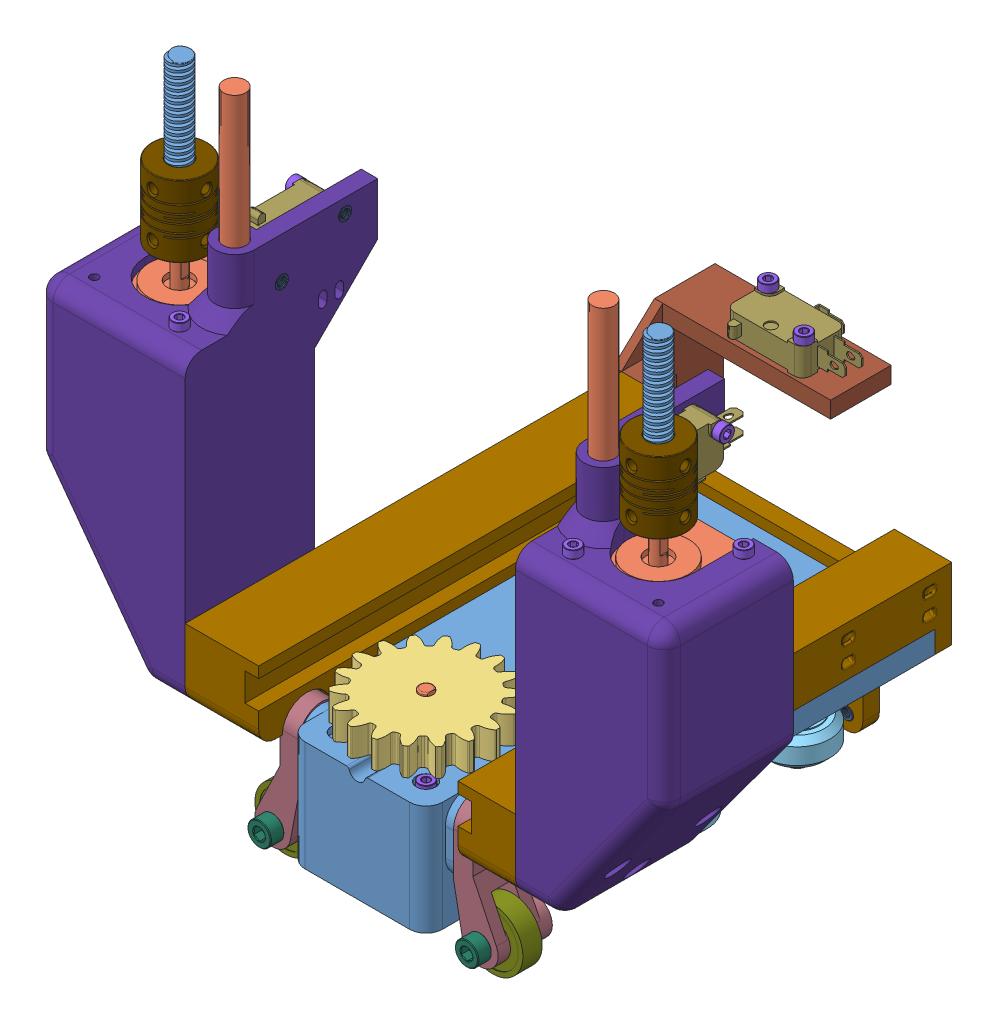
SolidWorks assembly SubAss_X_Carriage, configuration Default. Lengths in mm.
Overall size (285.53 295.94 195.55).
98 component instances, 20 part files, 108 mates.
Components (placement in the parent):
- X_Carriage-1: X_Carriage [Default] x (0 0 1) z (1 0 0) size (150 40 120)
- Nema17-1: Nema17 [Default] at (0 -16 65) x (-1 0 0) z (0 0 -1) size (42 55.32 47)
- Y_Pinion-1: Y_Pinion [Default] at (0 13 65) x (0.998835 0 -0.048265) z (0 -1 0) size (50 49.43 18)
- X_V_Wheel_spacer-1: X_V_Wheel_spacer [Default] at (45 -12.0098 19.85) size (8 8.02 8)
- Vslot_wheel-1: Vslot_wheel [Default] at (45 -21.5196 19.85) x (0 -1 0) z (0.174076 0 0.984732) size (11 23.9 23.9)
- 6_32_screw-1: 6_32_screw [6-32 Screw] at (45 -30.4 19.85) x (0.42455 0 0.905404) z (0 1 0) size (6.86 6.86 27.93)
- 6_32_locknut-1: 6_32_locknut [Default] at (45 -27.0196 19.85) x (-0.968538 0 -0.248866) z (-0.248866 0 0.968538) size (7.94 4.48 9.17)
- 6_32_locknut-2: 6_32_locknut [Default] at (45 -27.0196 -24.85) x (0.888394 0 -0.459082) z (-0.459082 0 -0.888394) size (7.94 4.48 9.17)
- 6_32_screw-2: 6_32_screw [6-32 Screw] at (45 -30.4 -24.85) x (-0.837169 0 -0.546944) z (0 1 0) size (6.86 6.86 27.93)
- Vslot_wheel-5: Vslot_wheel [Default] at (45 -21.5196 -24.85) x (0 -1 0) z (0.999776 0 -0.021145) size (11 23.9 23.9)
- X_V_Wheel_spacer-5: X_V_Wheel_spacer [Default] at (45 -12.0098 -24.85) x (0.954681 0 0.29763) z (-0.29763 0 0.954681) size (8 8.02 8)
- X_V_Wheel_spacer-6: X_V_Wheel_spacer [Default] at (-45 -12.0098 -24.85) x (-0.954681 0 0.29763) z (-0.29763 0 -0.954681) size (8 8.02 8)
- Vslot_wheel-6: Vslot_wheel [Default] at (-45 -21.5196 19.85) x (0 -1 0) z (0.174076 0 -0.984732) size (11 23.9 23.9)
- 6_32_screw-3: 6_32_screw [6-32 Screw] at (-45 -30.4 19.85) x (0.42455 0 -0.905404) z (0 1 0) size (6.86 6.86 27.93)
- 6_32_locknut-3: 6_32_locknut [Default] at (-45 -27.0196 19.85) x (-0.968538 0 0.248866) z (0.248866 0 0.968538) size (7.94 4.48 9.17)
- 6_32_locknut-4: 6_32_locknut [Default] at (-45 -27.0196 -24.85) x (0.888394 0 0.459082) z (0.459082 0 -0.888394) size (7.94 4.48 9.17)
- 6_32_screw-4: 6_32_screw [6-32 Screw] at (-45 -30.4 -24.85) x (0.837169 0 -0.546944) z (0 1 0) size (6.86 6.86 27.93)
- Vslot_wheel-7: Vslot_wheel [Default] at (-45 -21.5196 -24.85) x (0 -1 0) z (0.999776 0 0.021145) size (11 23.9 23.9)
- X_V_Wheel_spacer-7: X_V_Wheel_spacer [Default] at (-45 -12.0098 19.85) x (-1 0 0) z (0 0 -1) size (8 8.02 8)
- M3x12mm_screw-1: M3x12mm_screw [Default] at (-15.5 -14.4 49.5) x (-0.096062 0 -0.995375) z (0 -1 0) size (5.5 5.5 15.23)
- M3x12mm_screw-2: M3x12mm_screw [Default] at (15.5 -14.4 80.5) x (0.9313 0 0.364252) z (0 -1 0) size (5.5 5.5 15.23)
- Y_Support_rail-1: Y_Support_rail [Default] at (39.1416 14 0) x (-1 0 0) z (0 0 -1) size (120 66 158.55)
- M3x6mm_insert-1: M3x6mm_insert [Default] at (-44.2592 -0.9648 -44.9995) x (-1 0 0) z (0 0 1) size (4.85 6.68 4.85)
- M3x6mm_insert-2: M3x6mm_insert [Default] at (-44.2592 -0.9648 45.0005) x (-1 0 0) z (0 0 1) size (4.85 6.68 4.85)
- M3x6mm_insert-4: M3x6mm_insert [Default] at (-60.9648 11.4993 51.862) x (0 -0.381849 0.924225) z (0 -0.924225 -0.381849) size (4.85 6.68 4.85)
- M3x6mm_insert-5: M3x6mm_insert [Default] at (-60.9648 -1.5007 68.1391) x (0 -0.381849 0.924225) z (0 -0.924225 -0.381849) size (4.85 6.68 4.85)
- M3x6mm_insert-6: M3x6mm_insert [Default] at (-60.9648 11.4993 84.4162) x (0 -0.381849 0.924225) z (0 -0.924225 -0.381849) size (4.85 6.68 4.85)
- M3x6mm_insert-7: M3x6mm_insert [Default] at (-54.5006 12.4993 -66.9648) x (-0.923728 -0.383049 0) z (0.383049 -0.923728 0) size (4.85 6.68 4.85)
- M3x6mm_insert-8: M3x6mm_insert [Default] at (-54.5006 -2.5007 -66.9648) x (-0.923728 -0.383049 0) z (0.383049 -0.923728 0) size (4.85 6.68 4.85)
- M3x6mm_insert-9: M3x6mm_insert [Default] at (-27.8196 -6.0907 -66.9648) x (-0.923728 -0.383049 0) z (0.383049 -0.923728 0) size (4.85 6.68 4.85)
- M3x6mm_insert-10: M3x6mm_insert [Default] at (-27.8196 -42.396 -66.9648) x (-0.923728 -0.383049 0) z (0.383049 -0.923728 0) size (4.85 6.68 4.85)
- M3x6mm_insert-11: M3x6mm_insert [Default] at (-1.3506 -38.2207 -66.9648) x (-0.923728 -0.383049 0) z (0.383049 -0.923728 0) size (4.85 6.68 4.85)
- M3x6mm_insert-12: M3x6mm_insert [Default] at (-1.3506 -10.2807 -66.9648) x (-0.923728 -0.383049 0) z (0.383049 -0.923728 0) size (4.85 6.68 4.85)
- M3x6mm_insert-15: M3x6mm_insert [Default] at (60.9648 11.5001 51.8624) x (0 -0.381849 0.924225) z (0 0.924225 0.381849) size (4.85 6.68 4.85)
- M3x6mm_insert-16: M3x6mm_insert [Default] at (60.9648 -1.4999 68.1395) x (0 -0.381849 0.924225) z (0 0.924225 0.381849) size (4.85 6.68 4.85)
- M3x6mm_insert-17: M3x6mm_insert [Default] at (60.9648 11.5001 84.4165) x (0 -0.381849 0.924225) z (0 0.924225 0.381849) size (4.85 6.68 4.85)
- M3x6mm_insert-18: M3x6mm_insert [Default] at (27.8199 -6.0899 -66.9648) x (0.923728 -0.383049 0) z (0.383049 0.923728 0) size (4.85 6.68 4.85)
- M3x6mm_insert-19: M3x6mm_insert [Default] at (27.8199 -42.3952 -66.9648) x (0.923728 -0.383049 0) z (0.383049 0.923728 0) size (4.85 6.68 4.85)
- M3x6mm_insert-20: M3x6mm_insert [Default] at (-28.9648 -12.9992 75.0005) x (0 1 0) z (0 0 1) size (4.85 6.68 4.85)
- M3x6mm_insert-21: M3x6mm_insert [Default] at (28.9648 -13.0008 75.0005) x (0 -1 0) z (0 0 1) size (4.85 6.68 4.85)
- M3x12mm_screw-3: M3x12mm_screw [Default] at (-44.2584 6.4 -45) x (1 0 0) z (0 1 0) size (5.5 5.5 15.23)
- M3x12mm_screw-4: M3x12mm_screw [Default] at (-44.2584 6.4 45) x (1 0 0) z (0 1 0) size (5.5 5.5 15.23)
- M3x12mm_screw-9: M3x12mm_screw [Default] at (50.1416 6.4 -45) x (1 0 0) z (0 1 0) size (5.5 5.5 15.23)
- M3x12mm_screw-10: M3x12mm_screw [Default] at (50.1416 6.4 45) x (1 0 0) z (0 1 0) size (5.5 5.5 15.23)
- M3x6mm_insert-22: M3x6mm_insert [Default] at (50.1408 -0.9648 45.0005) x (-1 0 0) z (0 0 1) size (4.85 6.68 4.85)
- M3x6mm_insert-23: M3x6mm_insert [Default] at (50.1408 -0.9648 -44.9995) x (-1 0 0) z (0 0 1) size (4.85 6.68 4.85)
- Y_Switch_Bracket-1: Y_Switch_Bracket [Default] at (-54.5 5 -66) x (-1 0 0) z (0 0 -1) size (64 40 37)
- M3x6mm_insert-24: M3x6mm_insert [Default] at (-35.6978 32.9648 -95.0001) size (4.85 6.68 4.85)
- M3x6mm_insert-25: M3x6mm_insert [Default] at (-12.6978 32.9648 -85.0001) size (4.85 6.68 4.85)
- LimitSwitch-1: LimitSwitch [Default] at (-24.1986 37 -90.0006) x (1 0 0) z (0 -1 0) size (38 22 10)
- M3x12mm_screw-11: M3x12mm_screw [Default] at (-12.6986 30 -85.0006) x (1 0 0) z (0 -1 0) size (5.5 5.5 15.23)
- M3x12mm_screw-12: M3x12mm_screw [Default] at (-54.5 12.5 -60.6) size (5.5 5.5 15.23)
- M3x12mm_screw-13: M3x12mm_screw [Default] at (-54.5 -2.5 -60.6) size (5.5 5.5 15.23)
- M3x12mm_screw-14: M3x12mm_screw [Default] at (-35.6986 30 -95.0006) x (0.977997 0 -0.20862) z (0 -1 0) size (5.5 5.5 15.23)
- SubAss_Y_Wheel_Bracket-1: SubAss_Y_Wheel_Bracket [Symmetry] at (-28 -11.4203 75) size (22 51.02 25.55)
  - Y_Wheel_bracket-1: Y_Wheel_bracket [Symmetry] at origin size (16.19 46.52 19.7)
  - M5_nut-1: M5_nut [M5 Nut] at (-9.6915 -28.0196 -10) x (-0.866025 -0.5 0) z (-0.5 0.866025 0) size (8 4.62 9.24)
  - M5x16mm_screw-1: M5x16mm_screw [M5x16mm Screw] at (-9.6915 -28.0196 -8) x (-1 0 0) z (0 0 -1) size (8.5 8.5 21.45)
  - 608zz_ball_bearing-1: 608zz_ball_bearing [Défaut] at (-9.6915 -28.0196 0) x (0 0 -1) z (1 0 0) size (7 22 22)
- SubAss_Y_Wheel_Bracket-2: SubAss_Y_Wheel_Bracket [Default] at (28 -11.4203 75) size (22 51.02 25.55)
  - Y_Wheel_bracket-1: Y_Wheel_bracket [Default] at origin size (16.19 46.52 19.7)
  - M5_nut-1: M5_nut [M5 Nut] at (9.6915 -28.0196 -10) x (-0.866025 -0.5 0) z (-0.5 0.866025 0) size (8 4.62 9.24)
  - M5x16mm_screw-1: M5x16mm_screw [M5x16mm Screw] at (9.6915 -28.0196 -8) x (-1 0 0) z (0 0 -1) size (8.5 8.5 21.45)
  - 608zz_ball_bearing-1: 608zz_ball_bearing [Défaut] at (9.6915 -28.0196 0) x (0 0 -1) z (1 0 0) size (7 22 22)
- M3x12mm_screw-15: M3x12mm_screw [Default] at (23 -13 75) x (0 0 1) z (-1 0 0) size (5.5 5.5 15.23)
- M3x12mm_screw-16: M3x12mm_screw [Default] at (-23 -13 75) x (0 -0.904081 -0.427361) z (1 0 0) size (5.5 5.5 15.23)
- SubAss_Z_Motor_Bracket-1: SubAss_Z_Motor_Bracket [Default] at (73.8493 55.4563 -73.4458) size (119.14 279.71 167.01)
  - Z_Motor_bracket-1: Z_Motor_bracket [Default] at (13.1507 42.5437 141) x (0 0 1) z (-1 0 0) size (70 131 54)
  - Nema17-1: Nema17 [Default] at (13.1507 34.5437 141) x (-1 0 0) z (0 0 -1) size (42 55.32 47)
  - M3x12mm_screw-1: M3x12mm_screw [Default] at (-2.3493 33.5437 156.5) x (0.323816 0 -0.94612) z (0 -1 0) size (5.5 5.5 15.23)
  - M3x12mm_screw-2: M3x12mm_screw [Default] at (28.6507 33.5437 125.5) x (0.998238 0 0.059342) z (0 -1 0) size (5.5 5.5 15.23)
  - M3x12mm_screw-3: M3x12mm_screw [Default] at (-9.8493 52.5437 131) x (0 -0.297211 0.954812) z (-1 0 0) size (5.5 5.5 15.23)
  - M3x12mm_screw-4: M3x12mm_screw [Default] at (-9.8493 62.5437 108) x (0 -0.129774 0.991544) z (-1 0 0) size (5.5 5.5 15.23)
  - M3x6mm_insert-1: M3x6mm_insert [Default] at (-14.8141 52.5429 130.9995) x (0 -1 0) z (0 0 -1) size (4.85 6.68 4.85)
  - M3x6mm_insert-2: M3x6mm_insert [Default] at (-14.8141 62.5429 107.9995) x (0 -1 0) z (0 0 -1) size (4.85 6.68 4.85)
  - 5_to_8_mm_coupler-1: 5_to_8_mm_coupler [Default] at (13.1507 57.0437 141) size (20 26 20)
  - 8mm_leadscrew-1: 8mm_leadscrew [Default] at (13.1507 115.5437 141) x (-0.955094 0 0.296303) z (0 1 0) size (9.24 8.22 52.41)
  - 8mm_rod-1: 8mm_rod [Défaut] at (-6.8493 80.5437 141) x (0.883547 0 -0.468343) z (0.468343 0 0.883547) size (8 70 8)
  - LimitSwitch-1: LimitSwitch [Default] at (-2.8493 57.5437 119.5) x (0 0 -1) z (1 0 0) size (38 22 10)
- SubAss_Z_Motor_Bracket-2: SubAss_Z_Motor_Bracket [Symmetry] at (-46.1507 55.4563 -73.4458) size (165.53 279.71 167.01)
  - Z_Motor_bracket-1: Z_Motor_bracket [Symmetry] at (13.1507 42.5437 141) x (0 0 1) z (-1 0 0) size (70 131 54)
  - Nema17-1: Nema17 [Default] at (-40.8493 34.5437 141) x (-1 0 0) z (0 0 -1) size (42 55.32 47)
  - M3x12mm_screw-1: M3x12mm_screw [Default] at (-25.3493 33.5437 156.5) x (0.323816 0 -0.94612) z (0 -1 0) size (5.5 5.5 15.23)
  - M3x12mm_screw-2: M3x12mm_screw [Default] at (-56.3493 33.5437 125.5) x (0.998238 0 0.059342) z (0 -1 0) size (5.5 5.5 15.23)
  - M3x12mm_screw-3: M3x12mm_screw [Default] at (-17.8493 52.5437 131) x (0 0.99595 0.089904) z (1 0 0) size (5.5 5.5 15.23)
  - M3x12mm_screw-4: M3x12mm_screw [Default] at (-17.8493 62.5437 108) x (0 0.965963 0.25868) z (1 0 0) size (5.5 5.5 15.23)
  - M3x6mm_insert-1: M3x6mm_insert [Default] at (-12.653 52.5436 130.9991) x (0 0.381849 -0.924225) z (0 -0.924225 -0.381849) size (4.85 6.68 4.85)
  - M3x6mm_insert-2: M3x6mm_insert [Default] at (-12.653 62.5436 107.9991) x (0 0.381849 -0.924225) z (0 -0.924225 -0.381849) size (4.85 6.68 4.85)
  - 5_to_8_mm_coupler-1: 5_to_8_mm_coupler [Default] at (-40.8493 57.0437 141) size (20 26 20)
  - 8mm_leadscrew-1: 8mm_leadscrew [Default] at (-40.8493 115.5437 141) x (-0.955094 0 0.296303) z (0 1 0) size (9.24 8.22 52.41)
  - 8mm_rod-1: 8mm_rod [Défaut] at (-20.8493 80.5437 141) x (0.883547 0 -0.468343) z (0.468343 0 0.883547) size (8 70 8)
  - LimitSwitch-1: LimitSwitch [Default] at (-24.8493 57.5437 119.5) x (0 0 -1) z (1 0 0) size (38 22 10)
- M3x12mm_screw-17: M3x12mm_screw [Default] at (-56 11.5 51.8615) x (0 0 -1) z (1 0 0) size (5.5 5.5 15.23)
- M3x12mm_screw-18: M3x12mm_screw [Default] at (-56 -1.5 68.1385) x (0 -0.924225 -0.381849) z (1 0 0) size (5.5 5.5 15.23)
- M3x12mm_screw-19: M3x12mm_screw [Default] at (-56 11.5 84.4156) x (0 -0.924225 -0.381849) z (1 0 0) size (5.5 5.5 15.23)
- M3x12mm_screw-20: M3x12mm_screw [Default] at (56 11.5 84.4156) x (0 -0.924225 -0.381849) z (-1 0 0) size (5.5 5.5 15.23)
- M3x12mm_screw-21: M3x12mm_screw [Default] at (56 11.5 51.8615) x (0 0 -1) z (-1 0 0) size (5.5 5.5 15.23)
- M3x12mm_screw-22: M3x12mm_screw [Default] at (56 -1.5 68.1385) x (0 -0.924225 -0.381849) z (-1 0 0) size (5.5 5.5 15.23)
Mates (geometry in assembly coordinates):
- Coïncidente1: coincident aligned: plane of X_Carriage-1 through (0 0 0) normal (0 0 1)
- Coïncidente2: coincident anti-aligned: plane of X_Carriage-1 through (0 0 0) normal (0 -1 0)
- Coïncidente3: coincident aligned: plane of X_Carriage-1 through (0 0 0) normal (1 0 0)
- Coaxiale1: concentric anti-aligned: cylinder of X_Carriage-1 through (15.5 0 80.5) axis (0 1 0) radius 1.7; cylinder of Nema17-1 through (15.5 -8 80.5) axis (0 -1 0) radius 1.5
- Coaxiale2: concentric anti-aligned: cylinder of X_Carriage-1 through (-15.5 0 49.5) axis (0 1 0) radius 1.7; cylinder of Nema17-1 through (-15.5 -8 49.5) axis (0 -1 0) radius 1.5
- Coïncidente4: coincident anti-aligned: plane of X_Carriage-1 through (0 -8 0) normal (0 -1 0); plane of Nema17-1 through (0 -8 65) normal (0 1 0)
- Coaxiale3: concentric anti-aligned: cylinder of Nema17-1 through (0 14 65) axis (0 -1 0) radius 2.5; cylinder of Y_Pinion-1 through (0 -5 65) axis (0 1 0) radius 2.5
- Distance1: distance = 1 mm anti-aligned: plane of Y_Pinion-1 through (0 -5 65) normal (0 -1 0); plane of Nema17-1 through (0 -6 65) normal (0 1 0)
- Coaxiale4: concentric aligned: cylinder of X_Carriage-1 through (45 0 19.85) axis (0 -1 0) radius 1.85; cylinder of X_V_Wheel_spacer-1 through (45 -8 19.85) axis (0 -1 0) radius 4
- Coïncidente8: coincident anti-aligned: plane of X_Carriage-1 through (0 -8 0) normal (0 -1 0); plane of X_V_Wheel_spacer-1 through (45 -8 19.85) normal (0 1 0)
- Coaxiale5: concentric anti-aligned: cylinder of X_Carriage-1 through (45 -5 19.85) axis (0 1 0) radius 5.1; cylinder of 6_32_screw-1 through (45 -30.4 19.85) axis (0 -1 0) radius 3.429
- Coïncidente9: coincident anti-aligned: plane of X_Carriage-1 through (45 -5 19.85) normal (0 1 0); plane of 6_32_screw-1 through (45 -5 19.85) normal (0 -1 0)
- Coaxiale6: concentric anti-aligned: cylinder of X_V_Wheel_spacer-1 through (45 -8 19.85) axis (0 -1 0) radius 4; cylinder of Vslot_wheel-1 through (45 -27.0196 19.85) axis (0 1 0) radius 2.5
- Coïncidente10: coincident anti-aligned: plane of X_V_Wheel_spacer-1 through (45 -16.0196 19.85) normal (0 -1 0); plane of Vslot_wheel-1 through (45 -16.0196 19.85) normal (0 1 0)
- Coaxiale7: concentric aligned: circle of Vslot_wheel-1; circle of 6_32_locknut-1
- Coïncidente11: coincident anti-aligned: plane of Vslot_wheel-1 through (45 -27.0196 19.85) normal (0 -1 0); plane of 6_32_locknut-1 through (50.5546 -27.0196 14.1799) normal (0 1 0)
- Rainure1: slot aligned: cylinder of X_V_Wheel_spacer-5 through (45 -8 -24.85) axis (0 -1 0) radius 4; plane of X_Carriage-1 through (43.15 0 -24.85) normal (1 0 0); cylinder of X_Carriage-1 through (45 0 -24.85) axis (0 -1 0) radius 1.85
- Coaxiale8: concentric aligned: cylinder of 6_32_screw-2 through (45 -30.4 -24.85) axis (0 -1 0) radius 3.429; cylinder of X_V_Wheel_spacer-5 through (45 -8 -24.85) axis (0 -1 0) radius 2
- Coïncidente12: coincident anti-aligned: plane of X_Carriage-1 through (45 -5 -24.85) normal (0 1 0); plane of 6_32_screw-2 through (45 -5 -24.85) normal (0 -1 0)
- Coïncidente13: coincident anti-aligned: plane of X_Carriage-1 through (0 -8 0) normal (0 -1 0); plane of X_V_Wheel_spacer-5 through (45 -8 -24.85) normal (0 1 0)
- Coaxiale9: concentric anti-aligned: cylinder of Vslot_wheel-5 through (45 -27.0196 -24.85) axis (0 1 0) radius 2.5; cylinder of X_V_Wheel_spacer-5 through (45 -8 -24.85) axis (0 -1 0) radius 4
- Coïncidente14: coincident anti-aligned: plane of Vslot_wheel-5 through (45 -16.0196 -24.85) normal (0 1 0); plane of X_V_Wheel_spacer-5 through (45 -16.0196 -24.85) normal (0 -1 0)
- Coaxiale10: concentric aligned: circle of 6_32_locknut-2; cylinder of Vslot_wheel-5 through (45 -27.0196 -24.85) axis (0 1 0) radius 2.5
- Coïncidente15: coincident anti-aligned: plane of 6_32_locknut-2 through (44.6299 -27.0196 -16.9211) normal (0 1 0); plane of Vslot_wheel-5 through (45 -27.0196 -24.85) normal (0 -1 0)
- Coaxiale11: concentric anti-aligned: cylinder of X_Carriage-1 through (-15.5 0 49.5) axis (0 1 0) radius 3.5; cylinder of M3x12mm_screw-1 through (-15.5 0.6 49.5) axis (0 -1 0) radius 2.75
- Coaxiale12: concentric anti-aligned: cylinder of X_Carriage-1 through (15.5 0 80.5) axis (0 1 0) radius 3.5; cylinder of M3x12mm_screw-2 through (15.5 0.6 80.5) axis (0 -1 0) radius 2.75
- Coïncidente16: coincident anti-aligned: circle of X_Carriage-1; plane of M3x12mm_screw-2 through (15.5 -2.4 80.5) normal (0 -1 0)
- Coïncidente17: coincident anti-aligned: plane of X_Carriage-1 through (-15.5 -2.4 51.2) normal (0 1 0); plane of M3x12mm_screw-1 through (-15.5 -2.4 49.5) normal (0 -1 0)
- Coaxiale13: concentric aligned: cylinder of Y_Support_rail-1 through (-44.2584 0 -45) axis (0 -1 0) radius 2.25; cylinder of M3x6mm_insert-1 through (-44.2584 -1.9729 -45) axis (0 -1 0) radius 2.2215
- Coïncidente18: coincident aligned: plane of Y_Support_rail-1 through (-50.2584 0 -60) normal (0 -1 0); plane of M3x6mm_insert-1 through (-46.6523 0 -45) normal (0 -1 0)
- Coaxiale14: concentric aligned: cylinder of Y_Support_rail-1 through (-44.2584 0 45) axis (0 -1 0) radius 2.25; cylinder of M3x6mm_insert-2 through (-44.2584 -1.9729 45) axis (0 -1 0) radius 2.2215
- Coïncidente19: coincident aligned: plane of Y_Support_rail-1 through (-50.2584 0 -60) normal (0 -1 0); plane of M3x6mm_insert-2 through (-46.6523 0 45) normal (0 -1 0)
- Coaxiale15: concentric aligned: cylinder of Y_Support_rail-1 through (-60 11.5 51.8615) axis (-1 0 0) radius 2.25; cylinder of M3x6mm_insert-4 through (-61.9729 11.5 51.8615) axis (-1 0 0) radius 2.2215
- Coaxiale16: concentric aligned: cylinder of Y_Support_rail-1 through (-60 -1.5 68.1385) axis (-1 0 0) radius 2.25; cylinder of M3x6mm_insert-5 through (-61.9729 -1.5 68.1385) axis (-1 0 0) radius 2.2215
- Coaxiale17: concentric aligned: cylinder of Y_Support_rail-1 through (-60 11.5 84.4156) axis (-1 0 0) radius 2.25; cylinder of M3x6mm_insert-6 through (-61.9729 11.5 84.4156) axis (-1 0 0) radius 2.2215
- Coïncidente20: coincident aligned: plane of Y_Support_rail-1 through (-60 18 -66) normal (-1 0 0); plane of M3x6mm_insert-6 through (-60 10.5859 86.6281) normal (-1 0 0)
- Coïncidente21: coincident aligned: plane of Y_Support_rail-1 through (-60 18 -66) normal (-1 0 0); plane of M3x6mm_insert-4 through (-60 10.5859 54.0739) normal (-1 0 0)
- Coïncidente22: coincident aligned: plane of Y_Support_rail-1 through (-60 18 -66) normal (-1 0 0); plane of M3x6mm_insert-5 through (-60 -2.4141 70.351) normal (-1 0 0)
- Coaxiale18: concentric aligned: cylinder of Y_Support_rail-1 through (-54.5 12.5 -66) axis (0 0 -1) radius 2.25; cylinder of M3x6mm_insert-7 through (-54.5 12.5 -67.9729) axis (0 0 -1) radius 2.2215
- Coïncidente23: coincident aligned: plane of Y_Support_rail-1 through (39.1416 14 -66) normal (0 0 -1); plane of M3x6mm_insert-7 through (-56.7113 11.583 -66) normal (0 0 -1)
- Coaxiale19: concentric aligned: cylinder of Y_Support_rail-1 through (-54.5 -2.5 -66) axis (0 0 -1) radius 2.25; cylinder of M3x6mm_insert-8 through (-54.5 -2.5 -67.9729) axis (0 0 -1) radius 2.2215
- Coïncidente24: coincident aligned: plane of Y_Support_rail-1 through (39.1416 14 -66) normal (0 0 -1); plane of M3x6mm_insert-8 through (-56.7113 -3.417 -66) normal (0 0 -1)
- Coaxiale20: concentric aligned: cylinder of Y_Support_rail-1 through (-27.819 -6.09 -66) axis (0 0 -1) radius 2.25; cylinder of M3x6mm_insert-9 through (-27.819 -6.09 -67.9729) axis (0 0 -1) radius 2.2215
- Coïncidente25: coincident aligned: plane of Y_Support_rail-1 through (39.1416 14 -66) normal (0 0 -1); plane of M3x6mm_insert-9 through (-30.0303 -7.007 -66) normal (0 0 -1)
- Coaxiale21: concentric aligned: circle of Y_Support_rail-1; cylinder of M3x6mm_insert-10 through (-27.819 -42.3953 -67.9729) axis (0 0 -1) radius 2.2215
- Coïncidente26: coincident aligned: plane of Y_Support_rail-1 through (39.1416 14 -66) normal (0 0 -1); plane of M3x6mm_insert-10 through (-30.0303 -43.3122 -66) normal (0 0 -1)
- Coaxiale22: concentric aligned: cylinder of Y_Support_rail-1 through (-1.35 -38.22 -66) axis (0 0 -1) radius 2.25; cylinder of M3x6mm_insert-11 through (-1.35 -38.22 -67.9729) axis (0 0 -1) radius 2.2215
- Coïncidente27: coincident aligned: plane of Y_Support_rail-1 through (39.1416 14 -66) normal (0 0 -1); plane of M3x6mm_insert-11 through (-3.5613 -39.137 -66) normal (0 0 -1)
- Coaxiale23: concentric aligned: cylinder of Y_Support_rail-1 through (-1.35 -10.28 -66) axis (0 0 -1) radius 2.25; cylinder of M3x6mm_insert-12 through (-1.35 -10.28 -67.9729) axis (0 0 -1) radius 2.2215
- Coïncidente28: coincident aligned: plane of Y_Support_rail-1 through (39.1416 14 -66) normal (0 0 -1); plane of M3x6mm_insert-12 through (-3.5613 -11.197 -66) normal (0 0 -1)
- Coaxiale24: concentric aligned: cylinder of X_Carriage-1 through (-44.2584 -8 45) axis (0 -1 0) radius 1.7; cylinder of Y_Support_rail-1 through (-44.2584 0 45) axis (0 -1 0) radius 2.25
- Coaxiale25: concentric aligned: cylinder of X_Carriage-1 through (50.1416 -8 -45) axis (0 -1 0) radius 1.7; cylinder of Y_Support_rail-1 through (50.1416 0 -45) axis (0 -1 0) radius 2.25
- Coïncidente29: coincident anti-aligned: plane of X_Carriage-1 through (0 0 0) normal (0 1 0); plane of Y_Support_rail-1 through (56.1416 0 -60) normal (0 -1 0)
- Coaxiale26: concentric anti-aligned: cylinder of X_Carriage-1 through (28 -13 75) axis (1 0 0) radius 2.25; cylinder of M3x6mm_insert-20 through (-29.9729 -13 75) axis (-1 0 0) radius 2.2215
- Coïncidente30: coincident anti-aligned: plane of X_Carriage-1 through (-28 -8 75) normal (-1 0 0); circle of M3x6mm_insert-20
- Coaxiale28: concentric anti-aligned: cylinder of X_Carriage-1 through (-44.2584 -8 -45) axis (0 -1 0) radius 3.5; cylinder of M3x12mm_screw-3 through (-44.2584 -8.6 -45) axis (0 1 0) radius 2.75
- Coaxiale29: concentric anti-aligned: cylinder of X_Carriage-1 through (-44.2584 -8 45) axis (0 -1 0) radius 3.5; cylinder of M3x12mm_screw-4 through (-44.2584 -8.6 45) axis (0 1 0) radius 2.75
- Coïncidente31: coincident anti-aligned: plane of X_Carriage-1 through (-44.2584 -5.6 46.7) normal (0 -1 0); plane of M3x12mm_screw-4 through (-44.2584 -5.6 45) normal (0 1 0)
- Coïncidente32: coincident anti-aligned: plane of X_Carriage-1 through (-44.2584 -5.6 -43.3) normal (0 -1 0); plane of M3x12mm_screw-3 through (-44.2584 -5.6 -45) normal (0 1 0)
- Coaxiale30: concentric anti-aligned: cylinder of X_Carriage-1 through (50.1416 -8 -45) axis (0 -1 0) radius 3.5; cylinder of M3x12mm_screw-9 through (50.1416 -8.6 -45) axis (0 1 0) radius 2.75
- Coïncidente33: coincident anti-aligned: plane of X_Carriage-1 through (50.1416 -5.6 -43.3) normal (0 -1 0); plane of M3x12mm_screw-9 through (50.1416 -5.6 -45) normal (0 1 0)
- Coaxiale31: concentric anti-aligned: cylinder of X_Carriage-1 through (50.1416 -8 45) axis (0 -1 0) radius 3.5; cylinder of M3x12mm_screw-10 through (50.1416 -8.6 45) axis (0 1 0) radius 2.75
- Coïncidente34: coincident anti-aligned: plane of X_Carriage-1 through (50.1416 -5.6 46.7) normal (0 -1 0); plane of M3x12mm_screw-10 through (50.1416 -5.6 45) normal (0 1 0)
- Coaxiale32: concentric aligned: cylinder of Y_Support_rail-1 through (50.1416 0 45) axis (0 -1 0) radius 2.25; cylinder of M3x6mm_insert-22 through (50.1416 -1.9729 45) axis (0 -1 0) radius 2.2215
- Coïncidente35: coincident aligned: plane of Y_Support_rail-1 through (56.1416 0 -60) normal (0 -1 0); plane of M3x6mm_insert-22 through (47.7477 0 45) normal (0 -1 0)
- Coïncidente36: coincident aligned: plane of Y_Support_rail-1 through (56.1416 0 -60) normal (0 -1 0); plane of M3x6mm_insert-23 through (47.7477 0 -45) normal (0 -1 0)
- Coaxiale33: concentric aligned: cylinder of Y_Support_rail-1 through (50.1416 0 -45) axis (0 -1 0) radius 2.25; cylinder of M3x6mm_insert-23 through (50.1416 -1.9729 -45) axis (0 -1 0) radius 2.2215
- Coaxiale34: concentric aligned: circle of Y_Support_rail-1; cylinder of Y_Switch_Bracket-1 through (-54.5 12.5 -75) axis (0 0 -1) radius 1.7
- Coaxiale35: concentric aligned: circle of Y_Support_rail-1; cylinder of Y_Switch_Bracket-1 through (-54.5 -2.5 -75) axis (0 0 -1) radius 1.7
- Coïncidente37: coincident anti-aligned: plane of Y_Support_rail-1 through (39.1416 14 -66) normal (0 0 -1); plane of Y_Switch_Bracket-1 through (-54.5 5 -66) normal (0 0 1)
- Coaxiale36: concentric aligned: cylinder of Y_Switch_Bracket-1 through (-35.6986 32 -95.0006) axis (0 1 0) radius 2.25; cylinder of M3x6mm_insert-24 through (-35.6986 33.9729 -95.0006) axis (0 1 0) radius 2.2215
- Coïncidente38: coincident aligned: plane of Y_Switch_Bracket-1 through (-54.5 32 -66) normal (0 1 0); plane of M3x6mm_insert-24 through (-33.3048 32 -95.0006) normal (0 1 0)
- Coaxiale37: concentric aligned: cylinder of Y_Switch_Bracket-1 through (-12.6986 32 -85.0006) axis (0 1 0) radius 2.25; cylinder of M3x6mm_insert-25 through (-12.6986 33.9729 -85.0006) axis (0 1 0) radius 2.2215
- Coïncidente39: coincident aligned: plane of Y_Switch_Bracket-1 through (-54.5 32 -66) normal (0 1 0); plane of M3x6mm_insert-25 through (-10.3048 32 -85.0006) normal (0 1 0)
- Coaxiale41: concentric aligned: cylinder of Y_Switch_Bracket-1 through (-12.6986 32 -85.0006) axis (0 1 0) radius 2.25; cylinder of LimitSwitch-1 through (-12.6986 32 -85.0006) axis (0 1 0) radius 1.5
- Coaxiale42: concentric aligned: cylinder of Y_Switch_Bracket-1 through (-35.6986 32 -95.0006) axis (0 1 0) radius 2.25; cylinder of LimitSwitch-1 through (-35.6986 32 -95.0006) axis (0 1 0) radius 1.5
- Coïncidente40: coincident anti-aligned: plane of Y_Switch_Bracket-1 through (-54.5 32 -66) normal (0 1 0); plane of LimitSwitch-1 through (-38.1986 32 -98.0006) normal (0 -1 0)
- Coaxiale43: concentric anti-aligned: cylinder of LimitSwitch-1 through (-12.6986 32 -85.0006) axis (0 1 0) radius 1.5; cylinder of M3x12mm_screw-11 through (-12.6986 45 -85.0006) axis (0 -1 0) radius 2.75
- Coaxiale44: concentric anti-aligned: cylinder of LimitSwitch-1 through (-35.6986 32 -95.0006) axis (0 1 0) radius 1.5; cylinder of M3x12mm_screw-14 through (-35.6986 45 -95.0006) axis (0 -1 0) radius 2.75
- Coïncidente41: coincident anti-aligned: plane of LimitSwitch-1 through (-38.1986 42 -98.0006) normal (0 1 0); plane of M3x12mm_screw-14 through (-35.6986 42 -95.0006) normal (0 -1 0)
- Coïncidente42: coincident anti-aligned: plane of LimitSwitch-1 through (-38.1986 42 -98.0006) normal (0 1 0); plane of M3x12mm_screw-11 through (-12.6986 42 -85.0006) normal (0 -1 0)
- Coaxiale45: concentric anti-aligned: cylinder of Y_Switch_Bracket-1 through (-54.5 -2.5 -75) axis (0 0 -1) radius 3.5; cylinder of M3x12mm_screw-13 through (-54.5 -2.5 -75.6) axis (0 0 1) radius 2.75
- Coïncidente43: coincident anti-aligned: plane of Y_Switch_Bracket-1 through (-56.2 -2.5 -72.6) normal (0 0 -1); plane of M3x12mm_screw-13 through (-54.5 -2.5 -72.6) normal (0 0 1)
- Coaxiale46: concentric anti-aligned: cylinder of Y_Switch_Bracket-1 through (-54.5 12.5 -75) axis (0 0 -1) radius 3.5; cylinder of M3x12mm_screw-12 through (-54.5 12.5 -75.6) axis (0 0 1) radius 2.75
- Coïncidente44: coincident anti-aligned: plane of Y_Switch_Bracket-1 through (-56.2 12.5 -72.6) normal (0 0 -1); plane of M3x12mm_screw-12 through (-54.5 12.5 -72.6) normal (0 0 1)
- Rainure2: slot aligned: cylinder of X_Carriage-1 through (28 -13 75) axis (1 0 0) radius 2.25; plane of SubAss_Y_Wheel_Bracket-2/Y_Wheel_bracket-1 through (35 -13.8703 73.3) normal (0 0 1); cylinder of SubAss_Y_Wheel_Bracket-2/Y_Wheel_bracket-1 through (35 -8.9703 75) axis (1 0 0) radius 1.7
- Rainure3: slot anti-aligned: cylinder of X_Carriage-1 through (28 -13 75) axis (1 0 0) radius 2.25; plane of SubAss_Y_Wheel_Bracket-1/Y_Wheel_bracket-1 through (-35 -13.8703 73.3) normal (0 0 1); cylinder of SubAss_Y_Wheel_Bracket-1/Y_Wheel_bracket-1 through (-35 -8.9703 75) axis (-1 0 0) radius 1.7
- Coïncidente45: coincident anti-aligned: plane of X_Carriage-1 through (-28 -8 75) normal (-1 0 0); plane of SubAss_Y_Wheel_Bracket-1/Y_Wheel_bracket-1 through (-28 -7.4203 75) normal (1 0 0)
- Coïncidente46: coincident aligned: plane of X_Carriage-1 through (-28 -8 83) normal (0 0 1); plane of SubAss_Y_Wheel_Bracket-1/Y_Wheel_bracket-1 through (-35 -7.4203 83) normal (0 0 1)
- Coïncidente47: coincident aligned: plane of X_Carriage-1 through (28 -8 83) normal (0 0 1); plane of SubAss_Y_Wheel_Bracket-2/Y_Wheel_bracket-1 through (35 -7.4203 83) normal (0 0 1)
- Coïncidente48: coincident anti-aligned: plane of X_Carriage-1 through (28 -8 75) normal (1 0 0); plane of SubAss_Y_Wheel_Bracket-2/Y_Wheel_bracket-1 through (28 -7.4203 75) normal (-1 0 0)
- Coïncidente50: coincident anti-aligned: line of SubAss_Y_Wheel_Bracket-1/Y_Wheel_bracket-1 through (-35 -7.4203 83) axis (1 0 0); line of SubAss_Y_Wheel_Bracket-2/Y_Wheel_bracket-1 through (35 -7.4203 83) axis (-1 0 0)
- Coaxiale47: concentric aligned: cylinder of X_Carriage-1 through (28 -13 75) axis (1 0 0) radius 2.25; cylinder of M3x12mm_screw-16 through (-38 -13 75) axis (1 0 0) radius 2.75
- Coaxiale48: concentric anti-aligned: circle of X_Carriage-1; cylinder of M3x12mm_screw-15 through (38 -13 75) axis (-1 0 0) radius 2.75
- Coïncidente51: coincident anti-aligned: plane of SubAss_Y_Wheel_Bracket-1/Y_Wheel_bracket-1 through (-35 -7.4203 75) normal (-1 0 0); plane of M3x12mm_screw-16 through (-35 -13 75) normal (1 0 0)
- Coïncidente52: coincident anti-aligned: plane of SubAss_Y_Wheel_Bracket-2/Y_Wheel_bracket-1 through (35 -7.4203 75) normal (1 0 0); plane of M3x12mm_screw-15 through (35 -13 75) normal (-1 0 0)
- Coaxiale49: concentric anti-aligned: cylinder of Y_Support_rail-1 through (60 11.5 51.8615) axis (1 0 0) radius 2.25; cylinder of SubAss_Z_Motor_Bracket-1/Z_Motor_bracket-1 through (114 11.5 51.8615) axis (-1 0 0) radius 1.5
- Coaxiale50: concentric anti-aligned: cylinder of Y_Support_rail-1 through (60 11.5 84.4156) axis (1 0 0) radius 2.25; cylinder of SubAss_Z_Motor_Bracket-1/Z_Motor_bracket-1 through (114 11.5 84.4156) axis (-1 0 0) radius 1.5
- Coïncidente53: coincident anti-aligned: plane of Y_Support_rail-1 through (60 0 -60) normal (1 0 0); plane of SubAss_Z_Motor_Bracket-1/Z_Motor_bracket-1 through (60 63 45.5542) normal (-1 0 0)
- Coaxiale51: concentric anti-aligned: cylinder of Y_Support_rail-1 through (-60 11.5 51.8615) axis (-1 0 0) radius 2.25; cylinder of SubAss_Z_Motor_Bracket-2/Z_Motor_bracket-1 through (-114 11.5 51.8615) axis (1 0 0) radius 1.5
- Coaxiale52: concentric anti-aligned: cylinder of Y_Support_rail-1 through (-60 11.5 84.4156) axis (-1 0 0) radius 2.25; cylinder of SubAss_Z_Motor_Bracket-2/Z_Motor_bracket-1 through (-114 11.5 84.4156) axis (1 0 0) radius 1.5
- Coïncidente54: coincident anti-aligned: plane of Y_Support_rail-1 through (-60 18 -66) normal (-1 0 0); plane of SubAss_Z_Motor_Bracket-2/Z_Motor_bracket-1 through (-60 63 45.5542) normal (1 0 0)
- Coaxiale53: concentric aligned: cylinder of SubAss_Z_Motor_Bracket-2/Z_Motor_bracket-1 through (-114 11.5 51.8615) axis (1 0 0) radius 4; cylinder of M3x12mm_screw-17 through (-71 11.5 51.8615) axis (1 0 0) radius 2.75
- Coaxiale54: concentric aligned: cylinder of SubAss_Z_Motor_Bracket-2/Z_Motor_bracket-1 through (-114 11.5 84.4156) axis (1 0 0) radius 4; cylinder of M3x12mm_screw-19 through (-71 11.5 84.4156) axis (1 0 0) radius 2.75
- Coaxiale55: concentric aligned: cylinder of SubAss_Z_Motor_Bracket-2/Z_Motor_bracket-1 through (-114 -1.5 68.1385) axis (1 0 0) radius 4; cylinder of M3x12mm_screw-18 through (-71 -1.5 68.1385) axis (1 0 0) radius 2.75
- Coïncidente55: coincident anti-aligned: plane of SubAss_Z_Motor_Bracket-2/Z_Motor_bracket-1 through (-68 11.5 51.8615) normal (-1 0 0); plane of M3x12mm_screw-17 through (-68 11.5 51.8615) normal (1 0 0)
- Coïncidente56: coincident anti-aligned: plane of SubAss_Z_Motor_Bracket-2/Z_Motor_bracket-1 through (-68 11.5 84.4156) normal (-1 0 0); plane of M3x12mm_screw-19 through (-68 11.5 84.4156) normal (1 0 0)
- Coïncidente57: coincident anti-aligned: plane of SubAss_Z_Motor_Bracket-2/Z_Motor_bracket-1 through (-68 -1.5 68.1385) normal (-1 0 0); plane of M3x12mm_screw-18 through (-68 -1.5 68.1385) normal (1 0 0)
